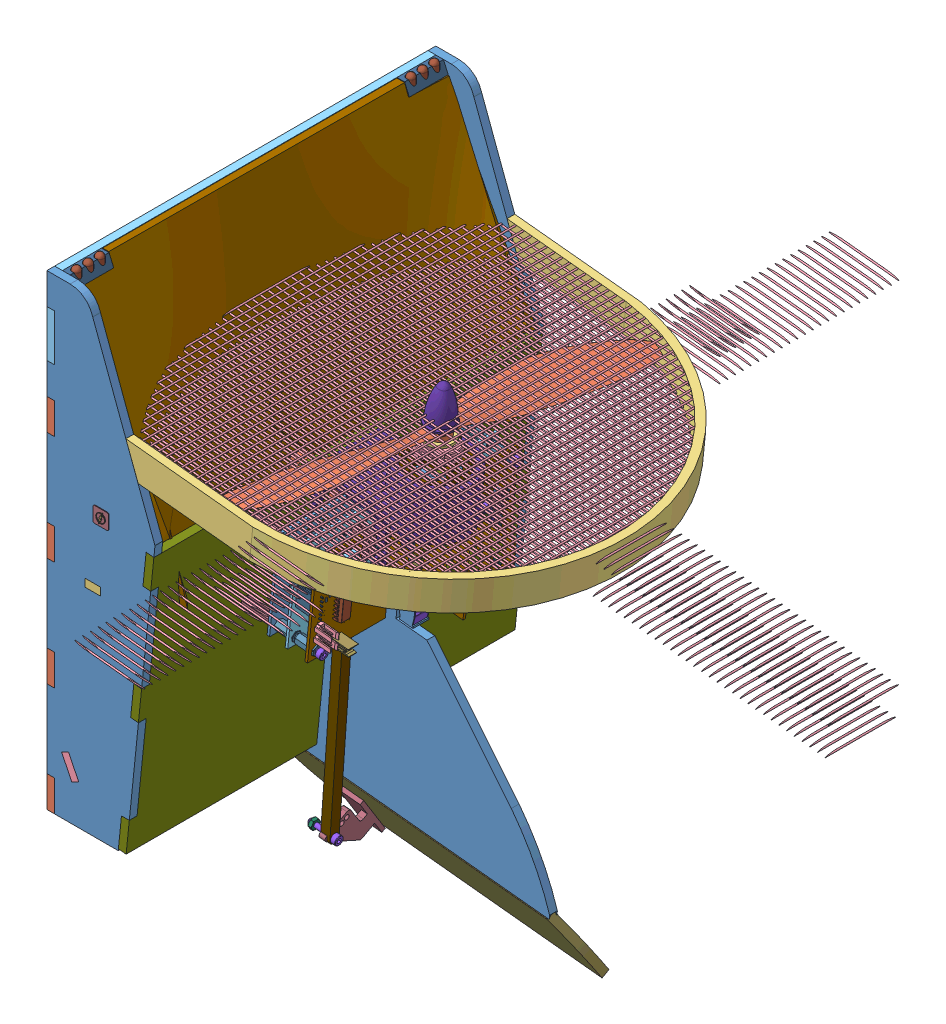
SolidWorks assembly AssTotaleSimu4, configuration Défaut. Lengths in mm. (continued)
Components (placement in the parent): (continued)
- AssStructSimu-1: AssStructSimu [Défaut] at (-125.7658 -1.8483 624.6548) x (1 0 0) z (0 0 -1) size (253.25 324.59 251.6) (continued)
  - AssProtec-1: AssProtec [Défaut] at (86.6746 190.4649 284.6351) x (0 0 -1) z (0.101852 -0.9948 0) size (250 237.46 20) (continued)
    - AssGrillage-2: AssGrillage [Défaut] at (339.6086 -132.5428 241.6839) x (0 0 1) z (-1 0 0) size (2.02 237.05 250) (continued)
      - barreau-208: barreau [Défaut] at (-0.1839 -1.5314 233.7823) x (0.998922 0 0.04641) z (0 1 0) size (1 1 400)
      - barreau-209: barreau [Défaut] at (-0.1839 -1.5314 228.7823) x (0.998922 0 0.04641) z (0 1 0) size (1 1 400)
      - barreau-210: barreau [Défaut] at (-0.1839 -1.5314 223.7823) x (0.998922 0 0.04641) z (0 1 0) size (1 1 400)
      - barreau-211: barreau [Défaut] at (-0.1839 -1.5314 218.7823) x (0.998922 0 0.04641) z (0 1 0) size (1 1 400)
      - barreau-212: barreau [Défaut] at (-0.1839 -1.5314 213.7823) x (0.998922 0 0.04641) z (0 1 0) size (1 1 400)
      - barreau-213: barreau [Défaut] at (-0.1839 -1.5314 208.7823) x (0.998922 0 0.04641) z (0 1 0) size (1 1 400)
      - barreau-214: barreau [Défaut] at (-0.1839 -1.5314 203.7823) x (0.998922 0 0.04641) z (0 1 0) size (1 1 400)
  - AssCarte-1: AssCarte [Défaut] at (38.0121 147.1029 290.772) x (-0.101852 0.9948 0) z (0.9948 0.101852 0) size (66.52 130.57 98.72)
    - carte_onduleur_v3-1: carte_onduleur_v3 [Défaut] at (-131.8199 12.0892 20.7912) size (66.52 130.57 82.34)
      - Layer_1-1: Layer_1 [Défaut] at origin size (60 130 1.61)
      - BTN-1: BTN [Défaut] at (-25.5 7.4 0.803) x (0 -1 0) z (0 0 1) size (6.76 3.64 4.37)
        - Open CASCADE STEP translator 6.8 1.2.1-1: Open CASCADE STEP translator 6.8 1.2.1 [Défaut] at origin size (6.76 3.64 4.37)
          - Body_1-1: Body_1 [Défaut] at (-0.5 -2 0) size (6.76 3.64 4.37)
            - =_[0_1_1_3]-1: =_[0_1_1_3] [Défaut] at origin size (6 3.64 4.37)
            - =_[0_1_1_4]-1: =_[0_1_1_4] [Défaut] at origin size (0.38 1 0.67)
            - =_[0_1_1_5]-1: =_[0_1_1_5] [Défaut] at origin size (0.38 1 0.67)
      - CON_IO1-1: CON_IO1 [Défaut] at (-11.3 12.1 0.803) x (0 -1 0) z (0 0 1) size (13 30 57.5)
        - Open CASCADE STEP translator 6.8 1.3.1-1: Open CASCADE STEP translator 6.8 1.3.1 [Défaut] at origin size (13 30 57.5)
          - Body_1_2-1: Body_1_2 [Défaut] at (-3 -15 8) x (0 -1 0) z (-1 0 0) size (30 57.5 13)
            - 1-1: 1 [Défaut] at origin size (30 50 1.61)
            - 10-1: 10 [Défaut] at (-14.395 31.0465 0.803) x (-1 0 0) z (0 0 1) size (5.59 6.35 1.11)
              - =_[0_1_1_4]-1: =_[0_1_1_4] [Défaut] at origin size (5.59 6.35 1.11)
                - 11-1: 11 [Défaut] at (2 3.3 0) x (-1 0 0) z (0 0 1) size (5.59 6.35 1.11)
                  - =_[0_1_1_3]_2-1: =_[0_1_1_3]_2 [Défaut] at origin size (0.44 0.55 0.36)
                  - =_[0_1_1_4]_2-1: =_[0_1_1_4]_2 [Défaut] at origin size (5.59 4.15 0.36)
                  - =_[0_1_1_5]_2-1: =_[0_1_1_5]_2 [Défaut] at origin size (5.35 6.1 1.1)
                  - =_[0_1_1_6]-1: =_[0_1_1_6] [Défaut] at origin size (0.44 0.55 0.36)
                  - =_[0_1_1_7]-1: =_[0_1_1_7] [Défaut] at origin size (0.44 0.55 0.36)
                  - =_[0_1_1_8]-1: =_[0_1_1_8] [Défaut] at origin size (0.44 0.55 0.36)
            - 13-1: 13 [Défaut] at (-12.62 16.6 -0.803) x (-1 0 0) z (0 0 -1) size (5.59 6.35 1.11)
              - =_[0_1_1_13]-1: =_[0_1_1_13] [Défaut] at origin size (5.59 6.35 1.11)
                - 11-1: 11 [Défaut] at (2 3.3 0) x (-1 0 0) z (0 0 1) size (5.59 6.35 1.11)
                  - =_[0_1_1_3]_2-1: =_[0_1_1_3]_2 [Défaut] at origin size (0.44 0.55 0.36)
                  - =_[0_1_1_4]_2-1: =_[0_1_1_4]_2 [Défaut] at origin size (5.59 4.15 0.36)
                  - =_[0_1_1_5]_2-1: =_[0_1_1_5]_2 [Défaut] at origin size (5.35 6.1 1.1)
                  - =_[0_1_1_6]-1: =_[0_1_1_6] [Défaut] at origin size (0.44 0.55 0.36)
                  - =_[0_1_1_7]-1: =_[0_1_1_7] [Défaut] at origin size (0.44 0.55 0.36)
                  - =_[0_1_1_8]-1: =_[0_1_1_8] [Défaut] at origin size (0.44 0.55 0.36)
            - 16-1: 16 [Défaut] at (-4.2 24.2 0.803) x (-1 0 0) z (0 0 1) size (12.8 0.5 13)
              - =_[0_1_1_15]-1: =_[0_1_1_15] [Défaut] at origin size (12.8 0.5 13)
                - 17-1: 17 [Défaut] at (2.7 0 0) x (1 0 0) z (0 -1 0) size (12.8 13 0.5)
            - 19-1: 19 [Défaut] at (-4.1 6.8 0.803) x (-1 0 0) z (0 0 1) size (12.8 0.5 13)
              - =_[0_1_1_18]-1: =_[0_1_1_18] [Défaut] at origin size (12.8 0.5 13)
                - 17-1: 17 [Défaut] at (2.7 0 0) x (1 0 0) z (0 -1 0) size (12.8 13 0.5)
            - 24-1: 24 [Défaut] at (-8.1 16.5 -0.803) x (0 1 0) z (0 0 -1) size (7.75 5.13 1.17)
              - =_[0_1_1_20]-1: =_[0_1_1_20] [Défaut] at origin size (7.75 5.13 1.17)
                - 20-1: 20 [Défaut] at origin size (7.59 5.13 1.07)
                - 21-1: 21 [Défaut] at (-14.478 0 0) x (-1 0 0) z (0 0 1) size (0.76 5.08 1.17)
                - 22-1: 22 [Défaut] at origin size (0.76 5.08 1.17)
            - 35-1: 35 [Défaut] at (-25.3 25.5 0.803) x (0 -1 0) z (0 0 1) size (6.05 5.2 1.7)
              - =_[0_1_1_25]-1: =_[0_1_1_25] [Défaut] at origin size (6.05 5.2 1.7)
                - 25-1: 25 [Défaut] at origin size (4.3 5.2 1.53)
                - 26-1: 26 [Défaut] at origin size (0.88 0.51 1.06)
                - 27-1: 27 [Défaut] at origin size (0.88 0.51 1.06)
                - 28-1: 28 [Défaut] at origin size (0.88 0.51 1.06)
                - 29-1: 29 [Défaut] at origin size (0.88 0.51 1.06)
                - 30-1: 30 [Défaut] at (11.6 -5.08 0) x (-1 0 0) z (0 0 1) size (0.87 0.51 1.06)
                - 31-1: 31 [Défaut] at (11.6 -2.54 0) x (-1 0 0) z (0 0 1) size (0.87 0.51 1.06)
                - 32-1: 32 [Défaut] at (11.6 0 0) x (-1 0 0) z (0 0 1) size (0.87 0.51 1.06)
                - 33-1: 33 [Défaut] at (11.6 2.54 0) x (-1 0 0) z (0 0 1) size (0.87 0.51 1.06)
            - 40-1: 40 [Défaut] at (-27.6 27.2 0.803) size (2.34 1.04 0.5)
              - =_[0_1_1_36]-1: =_[0_1_1_36] [Défaut] at origin size (2.34 1.04 0.5)
                - 36-1: 36 [Défaut] at origin size (2.29 1.04 0.43)
                - 37-1: 37 [Défaut] at (0.3048 0 0) x (-1 0 0) z (0 0 1) size (0.51 1.02 0.5)
                - 38-1: 38 [Défaut] at origin size (0.51 1.02 0.5)
            - 42-1: 42 [Défaut] at (-22.1 21.6 0.803) x (0 1 0) z (0 0 1) size (2.34 1.04 0.5)
              - =_[0_1_1_36]-1: =_[0_1_1_36] [Défaut] at origin size (2.34 1.04 0.5)
                - 36-1: 36 [Défaut] at origin size (2.29 1.04 0.43)
                - 37-1: 37 [Défaut] at (0.3048 0 0) x (-1 0 0) z (0 0 1) size (0.51 1.02 0.5)
                - 38-1: 38 [Défaut] at origin size (0.51 1.02 0.5)
            - 47-1: 47 [Défaut] at (-14.7664 14.5 -0.803) x (-1 0 0) z (0 0 -1) size (2.34 1.04 0.5)
              - =_[0_1_1_42]-1: =_[0_1_1_42] [Défaut] at origin size (2.34 1.04 0.5)
                - 43-1: 43 [Défaut] at origin size (2.29 1.04 0.43)
                - 44-1: 44 [Défaut] at (0.3048 0 0) x (-1 0 0) z (0 0 1) size (0.51 1.02 0.5)
                - 45-1: 45 [Défaut] at origin size (0.51 1.02 0.5)
            - 57-1: 57 [Défaut] at (-15.3 2.7 -0.803) x (0 -1 0) z (0 0 -1) size (10.36 15.24 6.14)
              - =_[0_1_1_47]-1: =_[0_1_1_47] [Défaut] at origin size (10.36 15.24 6.14)
                - 55-1: 55 [Défaut] at (1.8 -1.2 3) x (1 0 0) z (0 1 0) size (10.36 6.14 15.24)
                  - 54-1: 54 [Défaut] at origin size (10.36 6.14 7.62)
                    - 52-1: 52 [Défaut] at origin size (10.36 6.14 2.54)
                      - 48-1: 48 [Défaut] at origin size (8.4 2.54 2.54)
                      - 49-1: 49 [Défaut] at (-0.0461 1.2682 1.27) x (0 0 -1) z (0.999998 -0.002105 0) size (1.95 5.07 7.58)
                    - 52-2: 52 [Défaut] at (0 0 -2.54) size (10.36 6.14 2.54)
                      - 48-1: 48 [Défaut] at origin size (8.4 2.54 2.54)
                      - 49-1: 49 [Défaut] at (-0.0461 1.2682 1.27) x (0 0 -1) z (0.999998 -0.002105 0) size (1.95 5.07 7.58)
                    - 52-3: 52 [Défaut] at (0 0 -5.08) size (10.36 6.14 2.54)
                      - 48-1: 48 [Défaut] at origin size (8.4 2.54 2.54)
                      - 49-1: 49 [Défaut] at (-0.0461 1.2682 1.27) x (0 0 -1) z (0.999998 -0.002105 0) size (1.95 5.07 7.58)
                  - 54-2: 54 [Défaut] at (0 0 -7.62) size (10.36 6.14 7.62)
                    - 52-1: 52 [Défaut] at origin size (10.36 6.14 2.54)
                      - 48-1: 48 [Défaut] at origin size (8.4 2.54 2.54)
                      - 49-1: 49 [Défaut] at (-0.0461 1.2682 1.27) x (0 0 -1) z (0.999998 -0.002105 0) size (1.95 5.07 7.58)
                    - 52-2: 52 [Défaut] at (0 0 -2.54) size (10.36 6.14 2.54)
                      - 48-1: 48 [Défaut] at origin size (8.4 2.54 2.54)
                      - 49-1: 49 [Défaut] at (-0.0461 1.2682 1.27) x (0 0 -1) z (0.999998 -0.002105 0) size (1.95 5.07 7.58)
                    - 52-3: 52 [Défaut] at (0 0 -5.08) size (10.36 6.14 2.54)
                      - 48-1: 48 [Défaut] at origin size (8.4 2.54 2.54)
                      - 49-1: 49 [Défaut] at (-0.0461 1.2682 1.27) x (0 0 -1) z (0.999998 -0.002105 0) size (1.95 5.07 7.58)
            - 59-1: 59 [Défaut] at (-26.5 31 0.803) x (0 -1 0) z (0 0 1) size (2.34 1.04 0.5)
              - =_[0_1_1_42]-1: =_[0_1_1_42] [Défaut] at origin size (2.34 1.04 0.5)
                - 43-1: 43 [Défaut] at origin size (2.29 1.04 0.43)
                - 44-1: 44 [Défaut] at (0.3048 0 0) x (-1 0 0) z (0 0 1) size (0.51 1.02 0.5)
                - 45-1: 45 [Défaut] at origin size (0.51 1.02 0.5)
            - 61-1: 61 [Défaut] at (-21.6 17.8 0.803) x (-1 0 0) z (0 0 1) size (2.34 1.04 0.5)
              - =_[0_1_1_42]-1: =_[0_1_1_42] [Défaut] at origin size (2.34 1.04 0.5)
                - 43-1: 43 [Défaut] at origin size (2.29 1.04 0.43)
                - 44-1: 44 [Défaut] at (0.3048 0 0) x (-1 0 0) z (0 0 1) size (0.51 1.02 0.5)
                - 45-1: 45 [Défaut] at origin size (0.51 1.02 0.5)
            - 74-1: 74 [Défaut] at (-4.9 41.8 0.803) x (0 -1 0) z (0 0 1) size (6 4.9 1.75)
              - =_[0_1_1_56]-1: =_[0_1_1_56] [Défaut] at origin size (6 4.9 1.75)
                - 72-1: 72 [Défaut] at origin size (6 4.9 1.75)
                  - =_[0_1_1_2]-1: =_[0_1_1_2] [Défaut] at origin size (3.9 4.9 1.57)
                  - =_[0_1_1_3]-1: =_[0_1_1_3] [Défaut] at origin size (6 4.22 1)
                    - =_[0_1_1_60]-1: =_[0_1_1_60] [Défaut] at origin size (1.05 0.41 1)
                    - =_[0_1_1_61]-1: =_[0_1_1_61] [Défaut] at origin size (1.05 0.41 1)
                    - =_[0_1_1_62]-1: =_[0_1_1_62] [Défaut] at origin size (1.05 0.41 1)
                    - =_[0_1_1_63]-1: =_[0_1_1_63] [Défaut] at origin size (1.05 0.41 1)
                    - =_[0_1_1_64]-1: =_[0_1_1_64] [Défaut] at origin size (1.05 0.41 1)
                    - =_[0_1_1_65]-1: =_[0_1_1_65] [Défaut] at origin size (1.05 0.41 1)
                    - =_[0_1_1_66]-1: =_[0_1_1_66] [Défaut] at origin size (1.05 0.41 1)
                    - =_[0_1_1_67]-1: =_[0_1_1_67] [Défaut] at origin size (1.05 0.41 1)
            - 76-1: 76 [Défaut] at (-8.5 40.5664 0.803) x (0 1 0) z (0 0 1) size (2.34 1.04 0.5)
              - =_[0_1_1_42]-1: =_[0_1_1_42] [Défaut] at origin size (2.34 1.04 0.5)
                - 43-1: 43 [Défaut] at origin size (2.29 1.04 0.43)
                - 44-1: 44 [Défaut] at (0.3048 0 0) x (-1 0 0) z (0 0 1) size (0.51 1.02 0.5)
                - 45-1: 45 [Défaut] at origin size (0.51 1.02 0.5)
            - 78-1: 78 [Défaut] at (-5.9 46.4 0.803) x (-1 0 0) z (0 0 1) size (2.34 1.04 0.5)
              - =_[0_1_1_42]-1: =_[0_1_1_42] [Défaut] at origin size (2.34 1.04 0.5)
                - 43-1: 43 [Défaut] at origin size (2.29 1.04 0.43)
                - 44-1: 44 [Défaut] at (0.3048 0 0) x (-1 0 0) z (0 0 1) size (0.51 1.02 0.5)
                - 45-1: 45 [Défaut] at origin size (0.51 1.02 0.5)
            - 80-1: 80 [Défaut] at (-7 48.1 0.803) size (2.34 1.04 0.5)
              - =_[0_1_1_42]-1: =_[0_1_1_42] [Défaut] at origin size (2.34 1.04 0.5)
                - 43-1: 43 [Défaut] at origin size (2.29 1.04 0.43)
                - 44-1: 44 [Défaut] at (0.3048 0 0) x (-1 0 0) z (0 0 1) size (0.51 1.02 0.5)
                - 45-1: 45 [Défaut] at origin size (0.51 1.02 0.5)
            - 82-1: 82 [Défaut] at (-6 37.1 0.803) size (2.34 1.04 0.5)
              - =_[0_1_1_42]-1: =_[0_1_1_42] [Défaut] at origin size (2.34 1.04 0.5)
                - 43-1: 43 [Défaut] at origin size (2.29 1.04 0.43)
                - 44-1: 44 [Défaut] at (0.3048 0 0) x (-1 0 0) z (0 0 1) size (0.51 1.02 0.5)
                - 45-1: 45 [Défaut] at origin size (0.51 1.02 0.5)
      - CON_IO2-1: CON_IO2 [Défaut] at (-11.3 -2.7 0.803) x (0 -1 0) z (0 0 1) size (13 30 57.5)
        - Open CASCADE STEP translator 6.8 1.4.1-1: Open CASCADE STEP translator 6.8 1.4.1 [Défaut] at origin size (13 30 57.5)
          - Body_1_2-1: Body_1_2 [Défaut] at (-3 -15 8) x (0 -1 0) z (-1 0 0) size (30 57.5 13)
            - 1-1: 1 [Défaut] at origin size (30 50 1.61)
            - 10-1: 10 [Défaut] at (-14.395 31.0465 0.803) x (-1 0 0) z (0 0 1) size (5.59 6.35 1.11)
              - =_[0_1_1_4]-1: =_[0_1_1_4] [Défaut] at origin size (5.59 6.35 1.11)
                - 11-1: 11 [Défaut] at (2 3.3 0) x (-1 0 0) z (0 0 1) size (5.59 6.35 1.11)
                  - =_[0_1_1_3]_2-1: =_[0_1_1_3]_2 [Défaut] at origin size (0.44 0.55 0.36)
                  - =_[0_1_1_4]_2-1: =_[0_1_1_4]_2 [Défaut] at origin size (5.59 4.15 0.36)
                  - =_[0_1_1_5]_2-1: =_[0_1_1_5]_2 [Défaut] at origin size (5.35 6.1 1.1)
                  - =_[0_1_1_6]-1: =_[0_1_1_6] [Défaut] at origin size (0.44 0.55 0.36)
                  - =_[0_1_1_7]-1: =_[0_1_1_7] [Défaut] at origin size (0.44 0.55 0.36)
                  - =_[0_1_1_8]-1: =_[0_1_1_8] [Défaut] at origin size (0.44 0.55 0.36)
            - 13-1: 13 [Défaut] at (-12.62 16.6 -0.803) x (-1 0 0) z (0 0 -1) size (5.59 6.35 1.11)
              - =_[0_1_1_13]-1: =_[0_1_1_13] [Défaut] at origin size (5.59 6.35 1.11)
                - 11-1: 11 [Défaut] at (2 3.3 0) x (-1 0 0) z (0 0 1) size (5.59 6.35 1.11)
                  - =_[0_1_1_3]_2-1: =_[0_1_1_3]_2 [Défaut] at origin size (0.44 0.55 0.36)
                  - =_[0_1_1_4]_2-1: =_[0_1_1_4]_2 [Défaut] at origin size (5.59 4.15 0.36)
                  - =_[0_1_1_5]_2-1: =_[0_1_1_5]_2 [Défaut] at origin size (5.35 6.1 1.1)
                  - =_[0_1_1_6]-1: =_[0_1_1_6] [Défaut] at origin size (0.44 0.55 0.36)
                  - =_[0_1_1_7]-1: =_[0_1_1_7] [Défaut] at origin size (0.44 0.55 0.36)
                  - =_[0_1_1_8]-1: =_[0_1_1_8] [Défaut] at origin size (0.44 0.55 0.36)
            - 16-1: 16 [Défaut] at (-4.2 24.2 0.803) x (-1 0 0) z (0 0 1) size (12.8 0.5 13)
              - =_[0_1_1_15]-1: =_[0_1_1_15] [Défaut] at origin size (12.8 0.5 13)
                - 17-1: 17 [Défaut] at (2.7 0 0) x (1 0 0) z (0 -1 0) size (12.8 13 0.5)
            - 19-1: 19 [Défaut] at (-4.1 6.8 0.803) x (-1 0 0) z (0 0 1) size (12.8 0.5 13)
              - =_[0_1_1_18]-1: =_[0_1_1_18] [Défaut] at origin size (12.8 0.5 13)
                - 17-1: 17 [Défaut] at (2.7 0 0) x (1 0 0) z (0 -1 0) size (12.8 13 0.5)
            - 24-1: 24 [Défaut] at (-8.1 16.5 -0.803) x (0 1 0) z (0 0 -1) size (7.75 5.13 1.17)
              - =_[0_1_1_20]-1: =_[0_1_1_20] [Défaut] at origin size (7.75 5.13 1.17)
                - 20-1: 20 [Défaut] at origin size (7.59 5.13 1.07)
                - 21-1: 21 [Défaut] at (-14.478 0 0) x (-1 0 0) z (0 0 1) size (0.76 5.08 1.17)
                - 22-1: 22 [Défaut] at origin size (0.76 5.08 1.17)
            - 35-1: 35 [Défaut] at (-25.3 25.5 0.803) x (0 -1 0) z (0 0 1) size (6.05 5.2 1.7)
              - =_[0_1_1_25]-1: =_[0_1_1_25] [Défaut] at origin size (6.05 5.2 1.7)
                - 25-1: 25 [Défaut] at origin size (4.3 5.2 1.53)
                - 26-1: 26 [Défaut] at origin size (0.88 0.51 1.06)
                - 27-1: 27 [Défaut] at origin size (0.88 0.51 1.06)
                - 28-1: 28 [Défaut] at origin size (0.88 0.51 1.06)
                - 29-1: 29 [Défaut] at origin size (0.88 0.51 1.06)
                - 30-1: 30 [Défaut] at (11.6 -5.08 0) x (-1 0 0) z (0 0 1) size (0.87 0.51 1.06)
                - 31-1: 31 [Défaut] at (11.6 -2.54 0) x (-1 0 0) z (0 0 1) size (0.87 0.51 1.06)
                - 32-1: 32 [Défaut] at (11.6 0 0) x (-1 0 0) z (0 0 1) size (0.87 0.51 1.06)
                - 33-1: 33 [Défaut] at (11.6 2.54 0) x (-1 0 0) z (0 0 1) size (0.87 0.51 1.06)
            - 40-1: 40 [Défaut] at (-27.6 27.2 0.803) size (2.34 1.04 0.5)
              - =_[0_1_1_36]-1: =_[0_1_1_36] [Défaut] at origin size (2.34 1.04 0.5)
                - 36-1: 36 [Défaut] at origin size (2.29 1.04 0.43)
                - 37-1: 37 [Défaut] at (0.3048 0 0) x (-1 0 0) z (0 0 1) size (0.51 1.02 0.5)
                - 38-1: 38 [Défaut] at origin size (0.51 1.02 0.5)
            - 42-1: 42 [Défaut] at (-22.1 21.6 0.803) x (0 1 0) z (0 0 1) size (2.34 1.04 0.5)
              - =_[0_1_1_36]-1: =_[0_1_1_36] [Défaut] at origin size (2.34 1.04 0.5)
                - 36-1: 36 [Défaut] at origin size (2.29 1.04 0.43)
                - 37-1: 37 [Défaut] at (0.3048 0 0) x (-1 0 0) z (0 0 1) size (0.51 1.02 0.5)
                - 38-1: 38 [Défaut] at origin size (0.51 1.02 0.5)
            - 47-1: 47 [Défaut] at (-14.7664 14.5 -0.803) x (-1 0 0) z (0 0 -1) size (2.34 1.04 0.5)
              - =_[0_1_1_42]-1: =_[0_1_1_42] [Défaut] at origin size (2.34 1.04 0.5)
                - 43-1: 43 [Défaut] at origin size (2.29 1.04 0.43)
                - 44-1: 44 [Défaut] at (0.3048 0 0) x (-1 0 0) z (0 0 1) size (0.51 1.02 0.5)
                - 45-1: 45 [Défaut] at origin size (0.51 1.02 0.5)
            - 57-1: 57 [Défaut] at (-15.3 2.7 -0.803) x (0 -1 0) z (0 0 -1) size (10.36 15.24 6.14)
              - =_[0_1_1_47]-1: =_[0_1_1_47] [Défaut] at origin size (10.36 15.24 6.14)
                - 55-1: 55 [Défaut] at (1.8 -1.2 3) x (1 0 0) z (0 1 0) size (10.36 6.14 15.24)
                  - 54-1: 54 [Défaut] at origin size (10.36 6.14 7.62)
                    - 52-1: 52 [Défaut] at origin size (10.36 6.14 2.54)
                      - 48-1: 48 [Défaut] at origin size (8.4 2.54 2.54)
                      - 49-1: 49 [Défaut] at (-0.0461 1.2682 1.27) x (0 0 -1) z (0.999998 -0.002105 0) size (1.95 5.07 7.58)
                    - 52-2: 52 [Défaut] at (0 0 -2.54) size (10.36 6.14 2.54)
                      - 48-1: 48 [Défaut] at origin size (8.4 2.54 2.54)
                      - 49-1: 49 [Défaut] at (-0.0461 1.2682 1.27) x (0 0 -1) z (0.999998 -0.002105 0) size (1.95 5.07 7.58)
                    - 52-3: 52 [Défaut] at (0 0 -5.08) size (10.36 6.14 2.54)
                      - 48-1: 48 [Défaut] at origin size (8.4 2.54 2.54)
                      - 49-1: 49 [Défaut] at (-0.0461 1.2682 1.27) x (0 0 -1) z (0.999998 -0.002105 0) size (1.95 5.07 7.58)
                  - 54-2: 54 [Défaut] at (0 0 -7.62) size (10.36 6.14 7.62)
                    - 52-1: 52 [Défaut] at origin size (10.36 6.14 2.54)
                      - 48-1: 48 [Défaut] at origin size (8.4 2.54 2.54)
                      - 49-1: 49 [Défaut] at (-0.0461 1.2682 1.27) x (0 0 -1) z (0.999998 -0.002105 0) size (1.95 5.07 7.58)
                    - 52-2: 52 [Défaut] at (0 0 -2.54) size (10.36 6.14 2.54)
                      - 48-1: 48 [Défaut] at origin size (8.4 2.54 2.54)
                      - 49-1: 49 [Défaut] at (-0.0461 1.2682 1.27) x (0 0 -1) z (0.999998 -0.002105 0) size (1.95 5.07 7.58)
                    - 52-3: 52 [Défaut] at (0 0 -5.08) size (10.36 6.14 2.54)
                      - 48-1: 48 [Défaut] at origin size (8.4 2.54 2.54)
                      - 49-1: 49 [Défaut] at (-0.0461 1.2682 1.27) x (0 0 -1) z (0.999998 -0.002105 0) size (1.95 5.07 7.58)
            - 59-1: 59 [Défaut] at (-26.5 31 0.803) x (0 -1 0) z (0 0 1) size (2.34 1.04 0.5)
              - =_[0_1_1_42]-1: =_[0_1_1_42] [Défaut] at origin size (2.34 1.04 0.5)
                - 43-1: 43 [Défaut] at origin size (2.29 1.04 0.43)
                - 44-1: 44 [Défaut] at (0.3048 0 0) x (-1 0 0) z (0 0 1) size (0.51 1.02 0.5)
                - 45-1: 45 [Défaut] at origin size (0.51 1.02 0.5)
            - 61-1: 61 [Défaut] at (-21.6 17.8 0.803) x (-1 0 0) z (0 0 1) size (2.34 1.04 0.5)
              - =_[0_1_1_42]-1: =_[0_1_1_42] [Défaut] at origin size (2.34 1.04 0.5)
                - 43-1: 43 [Défaut] at origin size (2.29 1.04 0.43)
                - 44-1: 44 [Défaut] at (0.3048 0 0) x (-1 0 0) z (0 0 1) size (0.51 1.02 0.5)
                - 45-1: 45 [Défaut] at origin size (0.51 1.02 0.5)
            - 74-1: 74 [Défaut] at (-4.9 41.8 0.803) x (0 -1 0) z (0 0 1) size (6 4.9 1.75)
              - =_[0_1_1_56]-1: =_[0_1_1_56] [Défaut] at origin size (6 4.9 1.75)
                - 72-1: 72 [Défaut] at origin size (6 4.9 1.75)
                  - =_[0_1_1_2]-1: =_[0_1_1_2] [Défaut] at origin size (3.9 4.9 1.57)
                  - =_[0_1_1_3]-1: =_[0_1_1_3] [Défaut] at origin size (6 4.22 1)
                    - =_[0_1_1_60]-1: =_[0_1_1_60] [Défaut] at origin size (1.05 0.41 1)
                    - =_[0_1_1_61]-1: =_[0_1_1_61] [Défaut] at origin size (1.05 0.41 1)
                    - =_[0_1_1_62]-1: =_[0_1_1_62] [Défaut] at origin size (1.05 0.41 1)
                    - =_[0_1_1_63]-1: =_[0_1_1_63] [Défaut] at origin size (1.05 0.41 1)
                    - =_[0_1_1_64]-1: =_[0_1_1_64] [Défaut] at origin size (1.05 0.41 1)
                    - =_[0_1_1_65]-1: =_[0_1_1_65] [Défaut] at origin size (1.05 0.41 1)
                    - =_[0_1_1_66]-1: =_[0_1_1_66] [Défaut] at origin size (1.05 0.41 1)
                    - =_[0_1_1_67]-1: =_[0_1_1_67] [Défaut] at origin size (1.05 0.41 1)
            - 76-1: 76 [Défaut] at (-8.5 40.5664 0.803) x (0 1 0) z (0 0 1) size (2.34 1.04 0.5)
              - =_[0_1_1_42]-1: =_[0_1_1_42] [Défaut] at origin size (2.34 1.04 0.5)
                - 43-1: 43 [Défaut] at origin size (2.29 1.04 0.43)
                - 44-1: 44 [Défaut] at (0.3048 0 0) x (-1 0 0) z (0 0 1) size (0.51 1.02 0.5)
                - 45-1: 45 [Défaut] at origin size (0.51 1.02 0.5)
            - 78-1: 78 [Défaut] at (-5.9 46.4 0.803) x (-1 0 0) z (0 0 1) size (2.34 1.04 0.5)
              - =_[0_1_1_42]-1: =_[0_1_1_42] [Défaut] at origin size (2.34 1.04 0.5)
                - 43-1: 43 [Défaut] at origin size (2.29 1.04 0.43)
                - 44-1: 44 [Défaut] at (0.3048 0 0) x (-1 0 0) z (0 0 1) size (0.51 1.02 0.5)
                - 45-1: 45 [Défaut] at origin size (0.51 1.02 0.5)
            - 80-1: 80 [Défaut] at (-7 48.1 0.803) size (2.34 1.04 0.5)
              - =_[0_1_1_42]-1: =_[0_1_1_42] [Défaut] at origin size (2.34 1.04 0.5)
                - 43-1: 43 [Défaut] at origin size (2.29 1.04 0.43)
                - 44-1: 44 [Défaut] at (0.3048 0 0) x (-1 0 0) z (0 0 1) size (0.51 1.02 0.5)
                - 45-1: 45 [Défaut] at origin size (0.51 1.02 0.5)
            - 82-1: 82 [Défaut] at (-6 37.1 0.803) size (2.34 1.04 0.5)
              - =_[0_1_1_42]-1: =_[0_1_1_42] [Défaut] at origin size (2.34 1.04 0.5)
                - 43-1: 43 [Défaut] at origin size (2.29 1.04 0.43)
                - 44-1: 44 [Défaut] at (0.3048 0 0) x (-1 0 0) z (0 0 1) size (0.51 1.02 0.5)
                - 45-1: 45 [Défaut] at origin size (0.51 1.02 0.5)
      - CON_IO3-1: CON_IO3 [Défaut] at (-11.3 -17.7 0.803) x (0 -1 0) z (0 0 1) size (13 30 57.5)
        - Open CASCADE STEP translator 6.8 1.5.1-1: Open CASCADE STEP translator 6.8 1.5.1 [Défaut] at origin size (13 30 57.5)
          - Body_1_2-1: Body_1_2 [Défaut] at (-3 -15 8) x (0 -1 0) z (-1 0 0) size (30 57.5 13)
            - 1-1: 1 [Défaut] at origin size (30 50 1.61)
            - 10-1: 10 [Défaut] at (-14.395 31.0465 0.803) x (-1 0 0) z (0 0 1) size (5.59 6.35 1.11)
              - =_[0_1_1_4]-1: =_[0_1_1_4] [Défaut] at origin size (5.59 6.35 1.11)
                - 11-1: 11 [Défaut] at (2 3.3 0) x (-1 0 0) z (0 0 1) size (5.59 6.35 1.11)
                  - =_[0_1_1_3]_2-1: =_[0_1_1_3]_2 [Défaut] at origin size (0.44 0.55 0.36)
                  - =_[0_1_1_4]_2-1: =_[0_1_1_4]_2 [Défaut] at origin size (5.59 4.15 0.36)
                  - =_[0_1_1_5]_2-1: =_[0_1_1_5]_2 [Défaut] at origin size (5.35 6.1 1.1)
                  - =_[0_1_1_6]-1: =_[0_1_1_6] [Défaut] at origin size (0.44 0.55 0.36)
                  - =_[0_1_1_7]-1: =_[0_1_1_7] [Défaut] at origin size (0.44 0.55 0.36)
                  - =_[0_1_1_8]-1: =_[0_1_1_8] [Défaut] at origin size (0.44 0.55 0.36)
            - 13-1: 13 [Défaut] at (-12.62 16.6 -0.803) x (-1 0 0) z (0 0 -1) size (5.59 6.35 1.11)
              - =_[0_1_1_13]-1: =_[0_1_1_13] [Défaut] at origin size (5.59 6.35 1.11)
                - 11-1: 11 [Défaut] at (2 3.3 0) x (-1 0 0) z (0 0 1) size (5.59 6.35 1.11)
                  - =_[0_1_1_3]_2-1: =_[0_1_1_3]_2 [Défaut] at origin size (0.44 0.55 0.36)
                  - =_[0_1_1_4]_2-1: =_[0_1_1_4]_2 [Défaut] at origin size (5.59 4.15 0.36)
                  - =_[0_1_1_5]_2-1: =_[0_1_1_5]_2 [Défaut] at origin size (5.35 6.1 1.1)
                  - =_[0_1_1_6]-1: =_[0_1_1_6] [Défaut] at origin size (0.44 0.55 0.36)
                  - =_[0_1_1_7]-1: =_[0_1_1_7] [Défaut] at origin size (0.44 0.55 0.36)
                  - =_[0_1_1_8]-1: =_[0_1_1_8] [Défaut] at origin size (0.44 0.55 0.36)
            - 16-1: 16 [Défaut] at (-4.2 24.2 0.803) x (-1 0 0) z (0 0 1) size (12.8 0.5 13)
              - =_[0_1_1_15]-1: =_[0_1_1_15] [Défaut] at origin size (12.8 0.5 13)
                - 17-1: 17 [Défaut] at (2.7 0 0) x (1 0 0) z (0 -1 0) size (12.8 13 0.5)
            - 19-1: 19 [Défaut] at (-4.1 6.8 0.803) x (-1 0 0) z (0 0 1) size (12.8 0.5 13)
              - =_[0_1_1_18]-1: =_[0_1_1_18] [Défaut] at origin size (12.8 0.5 13)
                - 17-1: 17 [Défaut] at (2.7 0 0) x (1 0 0) z (0 -1 0) size (12.8 13 0.5)
            - 24-1: 24 [Défaut] at (-8.1 16.5 -0.803) x (0 1 0) z (0 0 -1) size (7.75 5.13 1.17)
              - =_[0_1_1_20]-1: =_[0_1_1_20] [Défaut] at origin size (7.75 5.13 1.17)
                - 20-1: 20 [Défaut] at origin size (7.59 5.13 1.07)
                - 21-1: 21 [Défaut] at (-14.478 0 0) x (-1 0 0) z (0 0 1) size (0.76 5.08 1.17)
                - 22-1: 22 [Défaut] at origin size (0.76 5.08 1.17)
            - 35-1: 35 [Défaut] at (-25.3 25.5 0.803) x (0 -1 0) z (0 0 1) size (6.05 5.2 1.7)
              - =_[0_1_1_25]-1: =_[0_1_1_25] [Défaut] at origin size (6.05 5.2 1.7)
                - 25-1: 25 [Défaut] at origin size (4.3 5.2 1.53)
                - 26-1: 26 [Défaut] at origin size (0.88 0.51 1.06)
                - 27-1: 27 [Défaut] at origin size (0.88 0.51 1.06)
                - 28-1: 28 [Défaut] at origin size (0.88 0.51 1.06)
                - 29-1: 29 [Défaut] at origin size (0.88 0.51 1.06)
                - 30-1: 30 [Défaut] at (11.6 -5.08 0) x (-1 0 0) z (0 0 1) size (0.87 0.51 1.06)
                - 31-1: 31 [Défaut] at (11.6 -2.54 0) x (-1 0 0) z (0 0 1) size (0.87 0.51 1.06)
                - 32-1: 32 [Défaut] at (11.6 0 0) x (-1 0 0) z (0 0 1) size (0.87 0.51 1.06)
                - 33-1: 33 [Défaut] at (11.6 2.54 0) x (-1 0 0) z (0 0 1) size (0.87 0.51 1.06)
            - 40-1: 40 [Défaut] at (-27.6 27.2 0.803) size (2.34 1.04 0.5)
              - =_[0_1_1_36]-1: =_[0_1_1_36] [Défaut] at origin size (2.34 1.04 0.5)
                - 36-1: 36 [Défaut] at origin size (2.29 1.04 0.43)
                - 37-1: 37 [Défaut] at (0.3048 0 0) x (-1 0 0) z (0 0 1) size (0.51 1.02 0.5)
                - 38-1: 38 [Défaut] at origin size (0.51 1.02 0.5)
            - 42-1: 42 [Défaut] at (-22.1 21.6 0.803) x (0 1 0) z (0 0 1) size (2.34 1.04 0.5)
              - =_[0_1_1_36]-1: =_[0_1_1_36] [Défaut] at origin size (2.34 1.04 0.5)
                - 36-1: 36 [Défaut] at origin size (2.29 1.04 0.43)
                - 37-1: 37 [Défaut] at (0.3048 0 0) x (-1 0 0) z (0 0 1) size (0.51 1.02 0.5)
                - 38-1: 38 [Défaut] at origin size (0.51 1.02 0.5)
            - 47-1: 47 [Défaut] at (-14.7664 14.5 -0.803) x (-1 0 0) z (0 0 -1) size (2.34 1.04 0.5)
              - =_[0_1_1_42]-1: =_[0_1_1_42] [Défaut] at origin size (2.34 1.04 0.5)
                - 43-1: 43 [Défaut] at origin size (2.29 1.04 0.43)
                - 44-1: 44 [Défaut] at (0.3048 0 0) x (-1 0 0) z (0 0 1) size (0.51 1.02 0.5)
                - 45-1: 45 [Défaut] at origin size (0.51 1.02 0.5)
            - 57-1: 57 [Défaut] at (-15.3 2.7 -0.803) x (0 -1 0) z (0 0 -1) size (10.36 15.24 6.14)
              - =_[0_1_1_47]-1: =_[0_1_1_47] [Défaut] at origin size (10.36 15.24 6.14)
                - 55-1: 55 [Défaut] at (1.8 -1.2 3) x (1 0 0) z (0 1 0) size (10.36 6.14 15.24)
                  - 54-1: 54 [Défaut] at origin size (10.36 6.14 7.62)
                    - 52-1: 52 [Défaut] at origin size (10.36 6.14 2.54)
                      - 48-1: 48 [Défaut] at origin size (8.4 2.54 2.54)
                      - 49-1: 49 [Défaut] at (-0.0461 1.2682 1.27) x (0 0 -1) z (0.999998 -0.002105 0) size (1.95 5.07 7.58)
                    - 52-2: 52 [Défaut] at (0 0 -2.54) size (10.36 6.14 2.54)
                      - 48-1: 48 [Défaut] at origin size (8.4 2.54 2.54)
                      - 49-1: 49 [Défaut] at (-0.0461 1.2682 1.27) x (0 0 -1) z (0.999998 -0.002105 0) size (1.95 5.07 7.58)
                    - 52-3: 52 [Défaut] at (0 0 -5.08) size (10.36 6.14 2.54)
                      - 48-1: 48 [Défaut] at origin size (8.4 2.54 2.54)
                      - 49-1: 49 [Défaut] at (-0.0461 1.2682 1.27) x (0 0 -1) z (0.999998 -0.002105 0) size (1.95 5.07 7.58)
                  - 54-2: 54 [Défaut] at (0 0 -7.62) size (10.36 6.14 7.62)
                    - 52-1: 52 [Défaut] at origin size (10.36 6.14 2.54)
                      - 48-1: 48 [Défaut] at origin size (8.4 2.54 2.54)
                      - 49-1: 49 [Défaut] at (-0.0461 1.2682 1.27) x (0 0 -1) z (0.999998 -0.002105 0) size (1.95 5.07 7.58)
                    - 52-2: 52 [Défaut] at (0 0 -2.54) size (10.36 6.14 2.54)
                      - 48-1: 48 [Défaut] at origin size (8.4 2.54 2.54)
                      - 49-1: 49 [Défaut] at (-0.0461 1.2682 1.27) x (0 0 -1) z (0.999998 -0.002105 0) size (1.95 5.07 7.58)
                    - 52-3: 52 [Défaut] at (0 0 -5.08) size (10.36 6.14 2.54)
                      - 48-1: 48 [Défaut] at origin size (8.4 2.54 2.54)
                      - 49-1: 49 [Défaut] at (-0.0461 1.2682 1.27) x (0 0 -1) z (0.999998 -0.002105 0) size (1.95 5.07 7.58)
            - 59-1: 59 [Défaut] at (-26.5 31 0.803) x (0 -1 0) z (0 0 1) size (2.34 1.04 0.5)
              - =_[0_1_1_42]-1: =_[0_1_1_42] [Défaut] at origin size (2.34 1.04 0.5)
                - 43-1: 43 [Défaut] at origin size (2.29 1.04 0.43)
                - 44-1: 44 [Défaut] at (0.3048 0 0) x (-1 0 0) z (0 0 1) size (0.51 1.02 0.5)
                - 45-1: 45 [Défaut] at origin size (0.51 1.02 0.5)
            - 61-1: 61 [Défaut] at (-21.6 17.8 0.803) x (-1 0 0) z (0 0 1) size (2.34 1.04 0.5)
              - =_[0_1_1_42]-1: =_[0_1_1_42] [Défaut] at origin size (2.34 1.04 0.5)
                - 43-1: 43 [Défaut] at origin size (2.29 1.04 0.43)
                - 44-1: 44 [Défaut] at (0.3048 0 0) x (-1 0 0) z (0 0 1) size (0.51 1.02 0.5)
                - 45-1: 45 [Défaut] at origin size (0.51 1.02 0.5)
            - 74-1: 74 [Défaut] at (-4.9 41.8 0.803) x (0 -1 0) z (0 0 1) size (6 4.9 1.75)
              - =_[0_1_1_56]-1: =_[0_1_1_56] [Défaut] at origin size (6 4.9 1.75)
                - 72-1: 72 [Défaut] at origin size (6 4.9 1.75)
                  - =_[0_1_1_2]-1: =_[0_1_1_2] [Défaut] at origin size (3.9 4.9 1.57)
                  - =_[0_1_1_3]-1: =_[0_1_1_3] [Défaut] at origin size (6 4.22 1)
                    - =_[0_1_1_60]-1: =_[0_1_1_60] [Défaut] at origin size (1.05 0.41 1)
                    - =_[0_1_1_61]-1: =_[0_1_1_61] [Défaut] at origin size (1.05 0.41 1)
                    - =_[0_1_1_62]-1: =_[0_1_1_62] [Défaut] at origin size (1.05 0.41 1)
                    - =_[0_1_1_63]-1: =_[0_1_1_63] [Défaut] at origin size (1.05 0.41 1)
                    - =_[0_1_1_64]-1: =_[0_1_1_64] [Défaut] at origin size (1.05 0.41 1)
                    - =_[0_1_1_65]-1: =_[0_1_1_65] [Défaut] at origin size (1.05 0.41 1)
                    - =_[0_1_1_66]-1: =_[0_1_1_66] [Défaut] at origin size (1.05 0.41 1)
                    - =_[0_1_1_67]-1: =_[0_1_1_67] [Défaut] at origin size (1.05 0.41 1)
            - 76-1: 76 [Défaut] at (-8.5 40.5664 0.803) x (0 1 0) z (0 0 1) size (2.34 1.04 0.5)
              - =_[0_1_1_42]-1: =_[0_1_1_42] [Défaut] at origin size (2.34 1.04 0.5)
                - 43-1: 43 [Défaut] at origin size (2.29 1.04 0.43)
                - 44-1: 44 [Défaut] at (0.3048 0 0) x (-1 0 0) z (0 0 1) size (0.51 1.02 0.5)
                - 45-1: 45 [Défaut] at origin size (0.51 1.02 0.5)
            - 78-1: 78 [Défaut] at (-5.9 46.4 0.803) x (-1 0 0) z (0 0 1) size (2.34 1.04 0.5)
              - =_[0_1_1_42]-1: =_[0_1_1_42] [Défaut] at origin size (2.34 1.04 0.5)
                - 43-1: 43 [Défaut] at origin size (2.29 1.04 0.43)
                - 44-1: 44 [Défaut] at (0.3048 0 0) x (-1 0 0) z (0 0 1) size (0.51 1.02 0.5)
                - 45-1: 45 [Défaut] at origin size (0.51 1.02 0.5)
            - 80-1: 80 [Défaut] at (-7 48.1 0.803) size (2.34 1.04 0.5)
              - =_[0_1_1_42]-1: =_[0_1_1_42] [Défaut] at origin size (2.34 1.04 0.5)
                - 43-1: 43 [Défaut] at origin size (2.29 1.04 0.43)
                - 44-1: 44 [Défaut] at (0.3048 0 0) x (-1 0 0) z (0 0 1) size (0.51 1.02 0.5)
                - 45-1: 45 [Défaut] at origin size (0.51 1.02 0.5)
            - 82-1: 82 [Défaut] at (-6 37.1 0.803) size (2.34 1.04 0.5)
              - =_[0_1_1_42]-1: =_[0_1_1_42] [Défaut] at origin size (2.34 1.04 0.5)
                - 43-1: 43 [Défaut] at origin size (2.29 1.04 0.43)
                - 44-1: 44 [Défaut] at (0.3048 0 0) x (-1 0 0) z (0 0 1) size (0.51 1.02 0.5)
                - 45-1: 45 [Défaut] at origin size (0.51 1.02 0.5)
      - C1_1-1: C1_1 [Défaut] at (-20.6336 6.4 -0.803) x (1 0 0) z (0 0 -1) size (2.34 1.04 0.5)
        - Open CASCADE STEP translator 6.8 1.6.1-1: Open CASCADE STEP translator 6.8 1.6.1 [Défaut] at origin size (2.34 1.04 0.5)
          - Body_1-1: Body_1 [Défaut] at origin size (2.29 1.04 0.43)
          - Pin_1-1: Pin_1 [Défaut] at (0.3048 0 0) x (-1 0 0) z (0 0 1) size (0.51 1.02 0.5)
          - Pin_2-1: Pin_2 [Défaut] at origin size (0.51 1.02 0.5)
      - C1_2-1: C1_2 [Défaut] at (-24.2 6.4 -0.803) x (1 0 0) z (0 0 -1) size (2.34 1.04 0.5)
        - Open CASCADE STEP translator 6.8 1.6.1-1: Open CASCADE STEP translator 6.8 1.6.1 [Défaut] at origin size (2.34 1.04 0.5)
          - Body_1-1: Body_1 [Défaut] at origin size (2.29 1.04 0.43)
          - Pin_1-1: Pin_1 [Défaut] at (0.3048 0 0) x (-1 0 0) z (0 0 1) size (0.51 1.02 0.5)
          - Pin_2-1: Pin_2 [Défaut] at origin size (0.51 1.02 0.5)
      - C_F-1: C_F [Défaut] at (-16.2432 4.45 -0.803) x (0 -1 0) z (0 0 -1) size (2.34 1.04 0.5)
        - Open CASCADE STEP translator 6.8 1.6.1-1: Open CASCADE STEP translator 6.8 1.6.1 [Défaut] at origin size (2.34 1.04 0.5)
          - Body_1-1: Body_1 [Défaut] at origin size (2.29 1.04 0.43)
          - Pin_1-1: Pin_1 [Défaut] at (0.3048 0 0) x (-1 0 0) z (0 0 1) size (0.51 1.02 0.5)
          - Pin_2-1: Pin_2 [Défaut] at origin size (0.51 1.02 0.5)
      - D_LED_STATE1-1: D_LED_STATE1 [Défaut] at (-6.8906 -21.6 0.803) size (2.34 1.04 0.5)
        - Open CASCADE STEP translator 6.8 1.6.1-1: Open CASCADE STEP translator 6.8 1.6.1 [Défaut] at origin size (2.34 1.04 0.5)
          - Body_1-1: Body_1 [Défaut] at origin size (2.29 1.04 0.43)
          - Pin_1-1: Pin_1 [Défaut] at (0.3048 0 0) x (-1 0 0) z (0 0 1) size (0.51 1.02 0.5)
          - Pin_2-1: Pin_2 [Défaut] at origin size (0.51 1.02 0.5)
      - PICKIT-1: PICKIT [Défaut] at (-24.1 -30.5 0.803) size (15.24 5 14.3)
        - Open CASCADE STEP translator 6.8 1.10.1-1: Open CASCADE STEP translator 6.8 1.10.1 [Défaut] at origin size (15.24 5 14.3)
          - Body_1_2-1: Body_1_2 [Défaut] at (6.3 0 12) size (15.24 5 14.3)
      - C_DEC_CUR-1: C_DEC_CUR [Défaut] at (-8.9496 5.7572 -0.803) x (0 1 0) z (0 0 -1) size (2.34 1.04 0.5)
        - Open CASCADE STEP translator 6.8 1.6.1-1: Open CASCADE STEP translator 6.8 1.6.1 [Défaut] at origin size (2.34 1.04 0.5)
          - Body_1-1: Body_1 [Défaut] at origin size (2.29 1.04 0.43)
          - Pin_1-1: Pin_1 [Défaut] at (0.3048 0 0) x (-1 0 0) z (0 0 1) size (0.51 1.02 0.5)
          - Pin_2-1: Pin_2 [Défaut] at origin size (0.51 1.02 0.5)
      - R_F-1: R_F [Défaut] at (-14.65 4.4432 -0.803) x (0 -1 0) z (0 0 -1) size (2.34 1.04 0.5)
        - Open CASCADE STEP translator 6.8 1.12.1-1: Open CASCADE STEP translator 6.8 1.12.1 [Défaut] at origin size (2.34 1.04 0.5)
          - Body_1_3-1: Body_1_3 [Défaut] at origin size (2.29 1.04 0.43)
          - Pin_1_2-1: Pin_1_2 [Défaut] at (0.3048 0 0) x (-1 0 0) z (0 0 1) size (0.51 1.02 0.5)
          - Pin_2_2-1: Pin_2_2 [Défaut] at origin size (0.51 1.02 0.5)
      - R_GAIN1-1: R_GAIN1 [Défaut] at (-13.95 5.7568 -0.803) x (0 1 0) z (0 0 -1) size (2.34 1.04 0.5)
        - Open CASCADE STEP translator 6.8 1.12.1-1: Open CASCADE STEP translator 6.8 1.12.1 [Défaut] at origin size (2.34 1.04 0.5)
          - Body_1_3-1: Body_1_3 [Défaut] at origin size (2.29 1.04 0.43)
          - Pin_1_2-1: Pin_1_2 [Défaut] at (0.3048 0 0) x (-1 0 0) z (0 0 1) size (0.51 1.02 0.5)
          - Pin_2_2-1: Pin_2_2 [Défaut] at origin size (0.51 1.02 0.5)
      - R_GAIN2-1: R_GAIN2 [Défaut] at (-15.65 7.9176 -0.803) x (0 -1 0) z (0 0 -1) size (2.34 1.04 0.5)
        - Open CASCADE STEP translator 6.8 1.12.1-1: Open CASCADE STEP translator 6.8 1.12.1 [Défaut] at origin size (2.34 1.04 0.5)
          - Body_1_3-1: Body_1_3 [Défaut] at origin size (2.29 1.04 0.43)
          - Pin_1_2-1: Pin_1_2 [Défaut] at (0.3048 0 0) x (-1 0 0) z (0 0 1) size (0.51 1.02 0.5)
          - Pin_2_2-1: Pin_2_2 [Défaut] at origin size (0.51 1.02 0.5)
      - R_LED_STATE1-1: R_LED_STATE1 [Défaut] at (-6.9242 -19.9 0.803) size (2.34 1.04 0.5)
        - Open CASCADE STEP translator 6.8 1.12.1-1: Open CASCADE STEP translator 6.8 1.12.1 [Défaut] at origin size (2.34 1.04 0.5)
          - Body_1_3-1: Body_1_3 [Défaut] at origin size (2.29 1.04 0.43)
          - Pin_1_2-1: Pin_1_2 [Défaut] at (0.3048 0 0) x (-1 0 0) z (0 0 1) size (0.51 1.02 0.5)
          - Pin_2_2-1: Pin_2_2 [Défaut] at origin size (0.51 1.02 0.5)
      - R_RESET1-1: R_RESET1 [Défaut] at (-23 7.9 0.803) size (2.34 1.04 0.5)
        - Open CASCADE STEP translator 6.8 1.12.1-1: Open CASCADE STEP translator 6.8 1.12.1 [Défaut] at origin size (2.34 1.04 0.5)
          - Body_1_3-1: Body_1_3 [Défaut] at origin size (2.29 1.04 0.43)
          - Pin_1_2-1: Pin_1_2 [Défaut] at (0.3048 0 0) x (-1 0 0) z (0 0 1) size (0.51 1.02 0.5)
          - Pin_2_2-1: Pin_2_2 [Défaut] at origin size (0.51 1.02 0.5)
